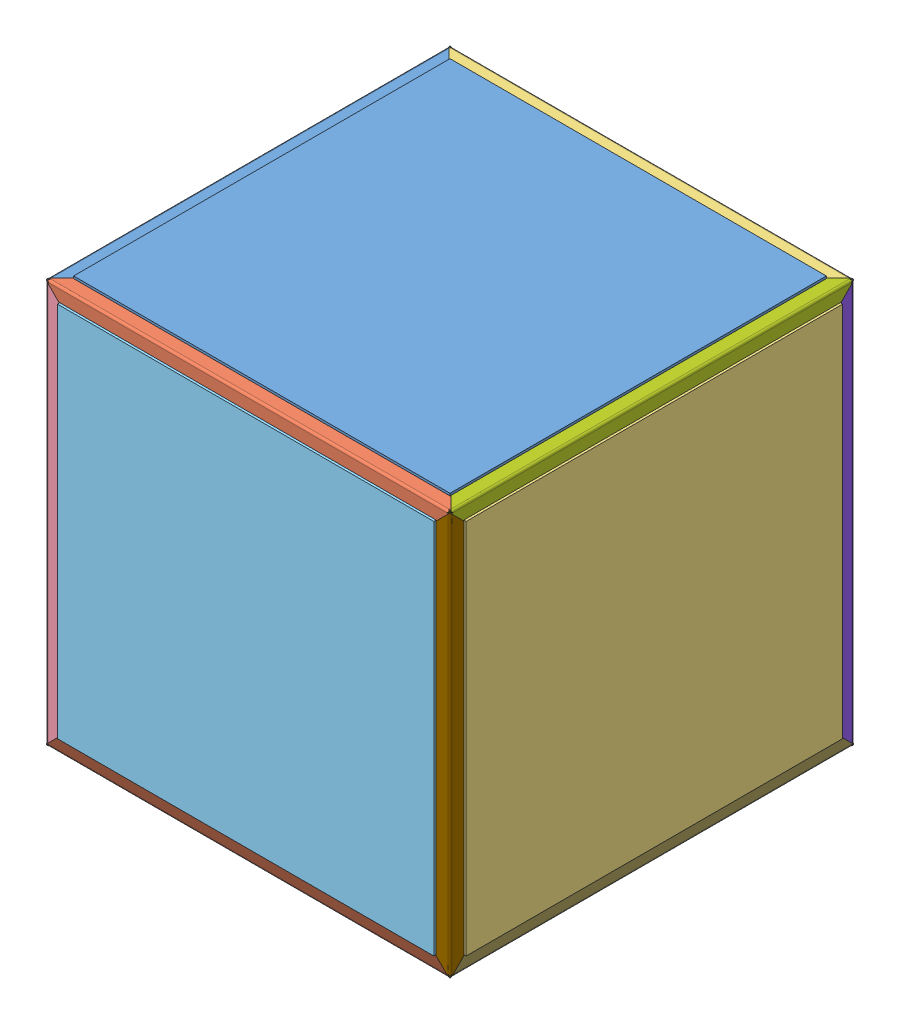
SolidWorks assembly cube_34, configuration cube34. Lengths in mm.
Overall size (280.03 280.03 280.03).
30 component instances, 30 part files, 93 mates.
Components (placement in the parent):
- pr^cube_34-28: pr^cube_34 [cube01] x (-1 0 0) z (0 0 1) size (257.81 1.59 257.81) (virtual)
- pg^cube_34-20: pg^cube_34 [cube01] x (0 -1 0) z (0 0 1) size (257.81 1.59 257.81) (virtual)
- po^cube_34-22: po^cube_34 [cube01] x (0 1 0) z (0 0 1) size (257.81 1.59 257.81) (virtual)
- py^cube_34-21: py^cube_34 [cube01] at origin size (257.81 1.59 257.81) (virtual)
- pc^cube_34-18: pc^cube_34 [cube01] x (-1 0 0) z (0 -1 0) size (257.81 1.59 257.81) (virtual)
- pb^cube_34-21: pb^cube_34 [cube01] x (-1 0 0) z (0 1 0) size (257.81 1.59 257.81) (virtual)
- br1^cube_34-49: br1^cube_34 [Default] at (0 113.03 -113.03) x (0 0 1) z (-1 0 0) size (50.8 50.8 218.95) (virtual)
- br2^cube_34-61: br2^cube_34 [Default] at (-113.03 113.03 0) size (50.8 50.8 218.95) (virtual)
- br3^cube_34-46: br3^cube_34 [Default] at (0 113.03 113.03) x (0 0 -1) z (1 0 0) size (50.8 50.8 218.95) (virtual)
- bg1^cube_34-47: bg1^cube_34 [Default] at (-113.03 -113.03 0) x (0 1 0) z (0 0 1) size (50.8 50.8 218.95) (virtual)
- bg2^cube_34-44: bg2^cube_34 [Default] at (-113.03 0 113.03) x (0 0 -1) z (0 1 0) size (50.8 50.8 218.95) (virtual)
- bg3^cube_34-40: bg3^cube_34 [Default] at (-113.03 0 -113.03) x (0 0 1) z (0 -1 0) size (50.8 50.8 218.95) (virtual)
- bo1^cube_34-42: bo1^cube_34 [Default] at (113.03 0 -113.03) x (0 0 1) z (0 1 0) size (50.8 50.8 218.95) (virtual)
- bo2^cube_34-46: bo2^cube_34 [Default] at (113.03 0 113.03) x (0 0 -1) z (0 -1 0) size (50.8 50.8 218.95) (virtual)
- bo3^cube_34-62: bo3^cube_34 [Default] at (113.03 113.03 0) x (0 -1 0) z (0 0 1) size (50.8 50.8 218.95) (virtual)
- by1^cube_34-41: by1^cube_34 [Default] at (0 -113.03 -113.03) x (0 0 1) z (1 0 0) size (50.8 50.8 218.95) (virtual)
- by2^cube_34-45: by2^cube_34 [Default] at (0 -113.03 113.03) x (0 0 -1) z (-1 0 0) size (50.8 50.8 218.95) (virtual)
- by3^cube_34-48: by3^cube_34 [Default] at (113.03 -113.03 0) x (-1 0 0) z (0 0 1) size (50.8 50.8 218.95) (virtual)
- dr1^cube_34-55: dr1^cube_34 [cube01] at (-137.8246 138.43 0) x (0 -1 0) z (0 0 1) size (26.01 26.01 276.87) (hidden, virtual)
- dr2^cube_34-37: dr2^cube_34 [cube01] at (0 138.43 137.8246) x (0 -1 0) z (1 0 0) size (26.01 26.01 276.87) (hidden, virtual)
- dr3^cube_34-33: dr3^cube_34 [cube01] at (0 138.43 -137.8246) x (0 -1 0) z (-1 0 0) size (26.01 26.01 276.87) (hidden, virtual)
- dg1^cube_34-38: dg1^cube_34 [cube01] at (-138.43 0 137.8246) x (1 0 0) z (0 1 0) size (26.01 26.01 276.87) (hidden, virtual)
- dg2^cube_34-41: dg2^cube_34 [cube01] at (-138.43 -137.8246 0) size (26.01 26.01 276.87) (hidden, virtual)
- dg3^cube_34-34: dg3^cube_34 [cube01] at (-138.43 0 -137.8246) x (1 0 0) z (0 -1 0) size (26.01 26.01 276.87) (hidden, virtual)
- do3^cube_34-47: do3^cube_34 [cube01] at (138.43 137.8246 0) x (-1 0 0) z (0 0 1) size (26.01 26.01 276.87) (hidden, virtual)
- do1^cube_34-36: do1^cube_34 [cube01] at (138.43 0 -137.8246) x (-1 0 0) z (0 1 0) size (26.01 26.01 276.87) (hidden, virtual)
- do2^cube_34-40: do2^cube_34 [cube01] at (138.43 0 137.8246) x (-1 0 0) z (0 -1 0) size (26.01 26.01 276.87) (hidden, virtual)
- dy1^cube_34-35: dy1^cube_34 [cube01] at (0 -138.43 -137.8246) x (0 1 0) z (1 0 0) size (26.01 26.01 276.87) (hidden, virtual)
- dy2^cube_34-39: dy2^cube_34 [cube01] at (0 -138.43 137.8246) x (0 1 0) z (-1 0 0) size (26.01 26.01 276.87) (hidden, virtual)
- dy3^cube_34-42: dy3^cube_34 [cube01] at (137.8246 -138.43 0) x (0 1 0) z (0 0 1) size (26.01 26.01 276.87) (hidden, virtual)
Mates (geometry in assembly coordinates):
- Coincident1: coincident anti-aligned: plane of pr^cube_34-28 through (128.905 138.43 -128.905) normal (0 -1 0); plane of br1^cube_34-49 through (-109.474 138.43 -113.03) normal (0 1 0)
- Coincident2: coincident anti-aligned: plane of pr^cube_34-28 through (128.905 138.43 -128.905) normal (0 -1 0); plane of br2^cube_34-61 through (-113.03 138.43 109.474) normal (0 1 0)
- Coincident3: coincident anti-aligned: plane of pr^cube_34-28 through (128.905 138.43 -128.905) normal (0 -1 0); plane of br3^cube_34-46 through (109.474 138.43 113.03) normal (0 1 0)
- Coincident4: coincident anti-aligned: plane of pr^cube_34-28 through (128.905 138.43 -128.905) normal (0 -1 0); plane of bo3^cube_34-62 through (113.03 138.43 109.474) normal (0 1 0)
- Coincident5: coincident anti-aligned: plane of pr^cube_34-28 through (128.905 138.43 -128.905) normal (0 -1 0); plane of dr3^cube_34-33 through (0 138.43 -276.2546) normal (0 1 0)
- Coincident6: coincident anti-aligned: plane of pr^cube_34-28 through (128.905 138.43 -128.905) normal (0 -1 0); plane of dr1^cube_34-55 through (-276.2546 138.43 0) normal (0 1 0)
- Coincident7: coincident anti-aligned: plane of pr^cube_34-28 through (128.905 138.43 -128.905) normal (0 -1 0); plane of do3^cube_34-47 through (-0.6054 138.43 0) normal (0 1 0)
- Coincident8: coincident anti-aligned: plane of pr^cube_34-28 through (128.905 138.43 -128.905) normal (0 -1 0); plane of dr2^cube_34-37 through (0 138.43 276.2546) normal (0 1 0)
- Coincident34: coincident anti-aligned: plane of pb^cube_34-21 through (128.905 -128.905 -138.43) normal (0 0 1); plane of by1^cube_34-41 through (109.474 -113.03 -138.43) normal (0 0 -1)
- Coincident35: coincident anti-aligned: plane of pb^cube_34-21 through (128.905 -128.905 -138.43) normal (0 0 1); plane of bo1^cube_34-42 through (113.03 109.474 -138.43) normal (0 0 -1)
- Coincident36: coincident anti-aligned: plane of pb^cube_34-21 through (128.905 -128.905 -138.43) normal (0 0 1); plane of br1^cube_34-49 through (-109.474 113.03 -138.43) normal (0 0 -1)
- Coincident37: coincident anti-aligned: plane of pb^cube_34-21 through (128.905 -128.905 -138.43) normal (0 0 1); plane of bg3^cube_34-40 through (-113.03 -109.474 -138.43) normal (0 0 -1)
- Coincident38: coincident anti-aligned: plane of pb^cube_34-21 through (128.905 -128.905 -138.43) normal (0 0 1); plane of dg3^cube_34-34 through (0.6054 0 -138.43) normal (0 0 -1)
- Coincident39: coincident anti-aligned: plane of pb^cube_34-21 through (128.905 -128.905 -138.43) normal (0 0 1); plane of dr3^cube_34-33 through (0 -0.6054 -138.43) normal (0 0 -1)
- Coincident40: coincident anti-aligned: plane of pb^cube_34-21 through (128.905 -128.905 -138.43) normal (0 0 1); plane of do1^cube_34-36 through (-0.6054 0 -138.43) normal (0 0 -1)
- Coincident41: coincident anti-aligned: plane of pb^cube_34-21 through (128.905 -128.905 -138.43) normal (0 0 1); plane of dy1^cube_34-35 through (0 0.6054 -138.43) normal (0 0 -1)
- Coincident42: coincident anti-aligned: plane of pc^cube_34-18 through (128.905 128.905 138.43) normal (0 0 -1); plane of bo2^cube_34-46 through (113.03 -109.474 138.43) normal (0 0 1)
- Coincident43: coincident anti-aligned: plane of pc^cube_34-18 through (128.905 128.905 138.43) normal (0 0 -1); plane of br3^cube_34-46 through (109.474 113.03 138.43) normal (0 0 1)
- Coincident44: coincident anti-aligned: plane of pc^cube_34-18 through (128.905 128.905 138.43) normal (0 0 -1); plane of bg2^cube_34-44 through (-113.03 109.474 138.43) normal (0 0 1)
- Coincident45: coincident anti-aligned: plane of pc^cube_34-18 through (128.905 128.905 138.43) normal (0 0 -1); plane of by2^cube_34-45 through (-109.474 -113.03 138.43) normal (0 0 1)
- Coincident46: coincident anti-aligned: plane of pc^cube_34-18 through (128.905 128.905 138.43) normal (0 0 -1); plane of do2^cube_34-40 through (-0.6054 0 138.43) normal (0 0 1)
- Coincident47: coincident anti-aligned: plane of pc^cube_34-18 through (128.905 128.905 138.43) normal (0 0 -1); plane of dy2^cube_34-39 through (0 0.6054 138.43) normal (0 0 1)
- Coincident48: coincident anti-aligned: plane of pc^cube_34-18 through (128.905 128.905 138.43) normal (0 0 -1); plane of dg1^cube_34-38 through (0.6054 0 138.43) normal (0 0 1)
- Coincident49: coincident anti-aligned: plane of pc^cube_34-18 through (128.905 128.905 138.43) normal (0 0 -1); plane of dr2^cube_34-37 through (0 -0.6054 138.43) normal (0 0 1)
- Coincident50: coincident anti-aligned: plane of pg^cube_34-20 through (-138.43 128.905 -128.905) normal (1 0 0); plane of bg3^cube_34-40 through (-138.43 -109.474 -113.03) normal (-1 0 0)
- Coincident51: coincident anti-aligned: plane of pg^cube_34-20 through (-138.43 128.905 -128.905) normal (1 0 0); plane of bg1^cube_34-47 through (-138.43 -113.03 109.474) normal (-1 0 0)
- Coincident52: coincident anti-aligned: plane of pg^cube_34-20 through (-138.43 128.905 -128.905) normal (1 0 0); plane of bg2^cube_34-44 through (-138.43 109.474 113.03) normal (-1 0 0)
- Coincident53: coincident anti-aligned: plane of pg^cube_34-20 through (-138.43 128.905 -128.905) normal (1 0 0); plane of dr1^cube_34-55 through (-138.43 -0.6054 0) normal (-1 0 0)
- Coincident54: coincident anti-aligned: plane of pg^cube_34-20 through (-138.43 128.905 -128.905) normal (1 0 0); plane of dg3^cube_34-34 through (-138.43 0 -276.2546) normal (-1 0 0)
- Coincident55: coincident anti-aligned: plane of pg^cube_34-20 through (-138.43 128.905 -128.905) normal (1 0 0); plane of dg2^cube_34-41 through (-138.43 -276.2546 0) normal (-1 0 0)
- Coincident56: coincident anti-aligned: plane of pg^cube_34-20 through (-138.43 128.905 -128.905) normal (1 0 0); plane of dg1^cube_34-38 through (-138.43 0 276.2546) normal (-1 0 0)
- Coincident99: coincident anti-aligned: plane of pg^cube_34-20 through (-138.43 128.905 -128.905) normal (1 0 0); plane of br2^cube_34-61 through (-138.43 113.03 109.474) normal (-1 0 0)
- Coincident57: coincident anti-aligned: plane of py^cube_34-21 through (-128.905 -138.43 -128.905) normal (0 1 0); plane of by3^cube_34-48 through (113.03 -138.43 109.474) normal (0 -1 0)
- Coincident58: coincident anti-aligned: plane of py^cube_34-21 through (-128.905 -138.43 -128.905) normal (0 1 0); plane of by2^cube_34-45 through (-109.474 -138.43 113.03) normal (0 -1 0)
- Coincident59: coincident anti-aligned: plane of py^cube_34-21 through (-128.905 -138.43 -128.905) normal (0 1 0); plane of bg1^cube_34-47 through (-113.03 -138.43 109.474) normal (0 -1 0)
- Coincident60: coincident anti-aligned: plane of py^cube_34-21 through (-128.905 -138.43 -128.905) normal (0 1 0); plane of by1^cube_34-41 through (109.474 -138.43 -113.03) normal (0 -1 0)
- Coincident61: coincident anti-aligned: plane of py^cube_34-21 through (-128.905 -138.43 -128.905) normal (0 1 0); plane of dy3^cube_34-42 through (276.2546 -138.43 0) normal (0 -1 0)
- Coincident62: coincident anti-aligned: plane of py^cube_34-21 through (-128.905 -138.43 -128.905) normal (0 1 0); plane of dy2^cube_34-39 through (0 -138.43 276.2546) normal (0 -1 0)
- Coincident63: coincident anti-aligned: plane of py^cube_34-21 through (-128.905 -138.43 -128.905) normal (0 1 0); plane of dg2^cube_34-41 through (0.6054 -138.43 0) normal (0 -1 0)
- Coincident64: coincident anti-aligned: plane of py^cube_34-21 through (-128.905 -138.43 -128.905) normal (0 1 0); plane of dy1^cube_34-35 through (0 -138.43 -276.2546) normal (0 -1 0)
- Coincident65: coincident anti-aligned: plane of po^cube_34-22 through (138.43 -128.905 -128.905) normal (-1 0 0); plane of bo1^cube_34-42 through (138.43 109.474 -113.03) normal (1 0 0)
- Coincident66: coincident anti-aligned: plane of po^cube_34-22 through (138.43 -128.905 -128.905) normal (-1 0 0); plane of by3^cube_34-48 through (138.43 -113.03 109.474) normal (1 0 0)
- Coincident67: coincident anti-aligned: plane of po^cube_34-22 through (138.43 -128.905 -128.905) normal (-1 0 0); plane of bo2^cube_34-46 through (138.43 -109.474 113.03) normal (1 0 0)
- Coincident68: coincident anti-aligned: plane of po^cube_34-22 through (138.43 -128.905 -128.905) normal (-1 0 0); plane of bo3^cube_34-62 through (138.43 113.03 109.474) normal (1 0 0)
- Coincident69: coincident anti-aligned: plane of po^cube_34-22 through (138.43 -128.905 -128.905) normal (-1 0 0); plane of do2^cube_34-40 through (138.43 0 276.2546) normal (1 0 0)
- Coincident70: coincident anti-aligned: plane of po^cube_34-22 through (138.43 -128.905 -128.905) normal (-1 0 0); plane of do3^cube_34-47 through (138.43 276.2546 0) normal (1 0 0)
- Coincident71: coincident anti-aligned: plane of po^cube_34-22 through (138.43 -128.905 -128.905) normal (-1 0 0); plane of do1^cube_34-36 through (138.43 0 -276.2546) normal (1 0 0)
- Coincident72: coincident anti-aligned: plane of po^cube_34-22 through (138.43 -128.905 -128.905) normal (-1 0 0); plane of dy3^cube_34-42 through (138.43 0.6054 0) normal (1 0 0)
- Coincident73: coincident aligned: plane of assembly through (0 0 0) normal (0 0 1); plane of dy3^cube_34-42 through (137.8246 -138.43 0) normal (0 0 1)
- Coincident74: coincident aligned: plane of assembly through (0 0 0) normal (0 0 1); plane of by3^cube_34-48 through (113.03 -113.03 0) normal (0 0 1)
- Coincident75: coincident aligned: plane of assembly through (0 0 0) normal (0 0 1); plane of bo3^cube_34-62 through (113.03 113.03 0) normal (0 0 1)
- Coincident76: coincident aligned: plane of assembly through (0 0 0) normal (0 0 1); plane of do3^cube_34-47 through (138.43 137.8246 0) normal (0 0 1)
- Coincident77: coincident aligned: plane of assembly through (0 0 0) normal (0 0 1); plane of dg2^cube_34-41 through (-138.43 -137.8246 0) normal (0 0 1)
- Coincident78: coincident aligned: plane of assembly through (0 0 0) normal (0 0 1); plane of bg1^cube_34-47 through (-113.03 -113.03 0) normal (0 0 1)
- Coincident79: coincident aligned: plane of assembly through (0 0 0) normal (0 0 1); plane of dr1^cube_34-55 through (-137.8246 138.43 0) normal (0 0 1)
- Coincident80: coincident aligned: plane of assembly through (0 0 0) normal (0 0 1); plane of br2^cube_34-61 through (-113.03 113.03 0) normal (0 0 1)
- Coincident81: coincident aligned: plane of assembly through (0 0 0) normal (0 1 0); plane of bo1^cube_34-42 through (113.03 0 -113.03) normal (0 1 0)
- Coincident82: coincident aligned: plane of assembly through (0 0 0) normal (0 1 0); plane of py^cube_34-21 through (0 0 0) normal (0 1 0)
- Coincident83: coincident aligned: plane of assembly through (0 0 0) normal (0 1 0); plane of do1^cube_34-36 through (138.43 0 -137.8246) normal (0 1 0)
- Coincident84: coincident anti-aligned: plane of assembly through (0 0 0) normal (0 1 0); plane of bg3^cube_34-40 through (-113.03 0 -113.03) normal (0 -1 0)
- Coincident85: coincident anti-aligned: plane of assembly through (0 0 0) normal (0 1 0); plane of dg3^cube_34-34 through (-138.43 0 -137.8246) normal (0 -1 0)
- Coincident86: coincident aligned: plane of assembly through (0 0 0) normal (0 1 0); plane of dg1^cube_34-38 through (-138.43 0 137.8246) normal (0 1 0)
- Coincident87: coincident aligned: plane of assembly through (0 0 0) normal (0 1 0); plane of bg2^cube_34-44 through (-113.03 0 113.03) normal (0 1 0)
- Coincident88: coincident anti-aligned: plane of assembly through (0 0 0) normal (0 1 0); plane of bo2^cube_34-46 through (113.03 0 113.03) normal (0 -1 0)
- Coincident89: coincident anti-aligned: plane of assembly through (0 0 0) normal (0 1 0); plane of do2^cube_34-40 through (138.43 0 137.8246) normal (0 -1 0)
- Coincident90: coincident anti-aligned: plane of assembly through (0 0 0) normal (1 0 0); plane of by2^cube_34-45 through (0 -113.03 113.03) normal (-1 0 0)
- Coincident91: coincident anti-aligned: plane of assembly through (0 0 0) normal (1 0 0); plane of dy2^cube_34-39 through (0 -138.43 137.8246) normal (-1 0 0)
- Coincident92: coincident aligned: plane of assembly through (0 0 0) normal (1 0 0); plane of pg^cube_34-20
- Coincident93: coincident aligned: plane of assembly through (0 0 0) normal (1 0 0); plane of dr2^cube_34-37 through (0 138.43 137.8246) normal (1 0 0)
- Coincident94: coincident aligned: plane of assembly through (0 0 0) normal (1 0 0); plane of br3^cube_34-46 through (0 113.03 113.03) normal (1 0 0)
- Coincident95: coincident anti-aligned: plane of assembly through (0 0 0) normal (1 0 0); plane of dr3^cube_34-33 through (0 138.43 -137.8246) normal (-1 0 0)
- Coincident96: coincident anti-aligned: plane of assembly through (0 0 0) normal (1 0 0); plane of br1^cube_34-49 through (0 113.03 -113.03) normal (-1 0 0)
- Coincident97: coincident aligned: plane of assembly through (0 0 0) normal (1 0 0); plane of by1^cube_34-41 through (0 -113.03 -113.03) normal (1 0 0)
- Coincident98: coincident aligned: plane of assembly through (0 0 0) normal (1 0 0); plane of dy1^cube_34-35 through (0 -138.43 -137.8246) normal (1 0 0)
- Coincident100: coincident anti-aligned: plane of pr^cube_34-28; plane of assembly through (0 0 0) normal (1 0 0)
- Coincident101: coincident aligned: plane of pr^cube_34-28 through (0 0 0) normal (0 0 1); plane of assembly through (0 0 0) normal (0 0 1)
- Coincident102: coincident anti-aligned: plane of pr^cube_34-28; plane of assembly through (0 0 0) normal (0 1 0)
- Coincident106: coincident anti-aligned: plane of pg^cube_34-20; plane of assembly through (0 0 0) normal (0 1 0)
- Coincident107: coincident aligned: plane of pg^cube_34-20; plane of assembly through (0 0 0) normal (1 0 0)
- Coincident108: coincident aligned: plane of pg^cube_34-20 through (0 0 0) normal (0 0 1); plane of assembly through (0 0 0) normal (0 0 1)
- Coincident109: coincident aligned: plane of py^cube_34-21 through (0 0 0) normal (0 0 1); plane of assembly through (0 0 0) normal (0 0 1)
- Coincident110: coincident aligned: plane of py^cube_34-21 through (0 0 0) normal (0 1 0); plane of assembly through (0 0 0) normal (0 1 0)
- Coincident111: coincident aligned: plane of py^cube_34-21 through (0 0 0) normal (1 0 0); plane of assembly through (0 0 0) normal (1 0 0)
- Coincident112: coincident aligned: plane of po^cube_34-22 through (0 0 0) normal (0 0 1); plane of assembly through (0 0 0) normal (0 0 1)
- Coincident113: coincident anti-aligned: plane of po^cube_34-22; plane of assembly through (0 0 0) normal (1 0 0)
- Coincident114: coincident aligned: plane of po^cube_34-22; plane of assembly through (0 0 0) normal (0 1 0)
- Coincident115: coincident anti-aligned: plane of pc^cube_34-18 through (0 0 0) normal (0 -1 0); plane of assembly through (0 0 0) normal (0 1 0)
- Coincident116: coincident anti-aligned: plane of pc^cube_34-18; plane of assembly through (0 0 0) normal (0 0 1)
- Coincident117: coincident anti-aligned: plane of pc^cube_34-18; plane of assembly through (0 0 0) normal (1 0 0)
- Coincident118: coincident aligned: plane of pb^cube_34-21 through (0 0 0) normal (0 1 0); plane of assembly through (0 0 0) normal (0 1 0)
- Coincident119: coincident aligned: plane of pb^cube_34-21; plane of assembly through (0 0 0) normal (0 0 1)
- Coincident120: coincident anti-aligned: line of pb^cube_34-21 through (0.8731 -0.8731 0) axis (0 0 -1); sketch_entity of pr^cube_34-28; plane of pb^cube_34-21 through (128.905 -128.905 -140.0175) normal (0 0 -1); plane of py^cube_34-21 through (-128.905 -140.0175 -128.905) normal (0 -1 0)
- cyan_cut: unknown: unknown of pc^cube_34-18; plane of pc^cube_34-18 through (128.905 128.905 140.0175) normal (0 0 1); plane of pg^cube_34-20 through (-140.0175 128.905 -128.905) normal (-1 0 0); plane of po^cube_34-22 through (140.0175 -128.905 -128.905) normal (1 0 0)
